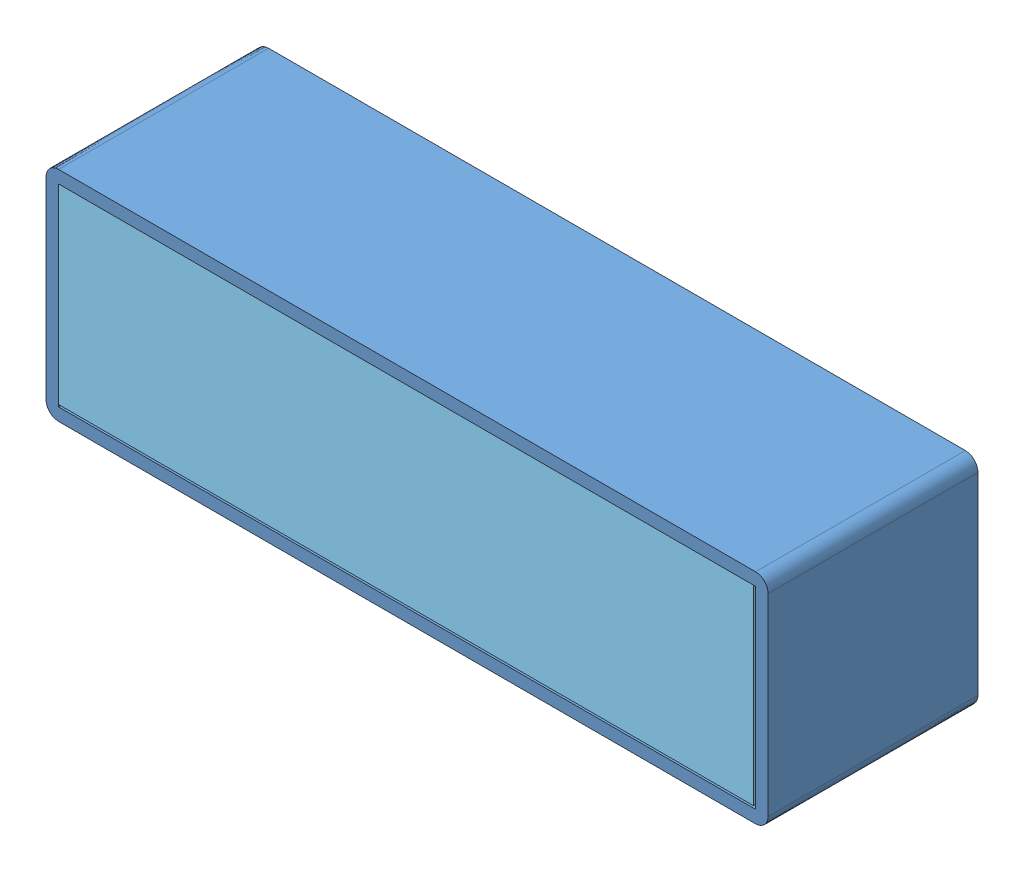
SolidWorks assembly miniAWTRIX, configuration Default. Lengths in mm.
Overall size (172 52 50).
7 component instances, 7 part files, 11 mates.
Components (placement in the parent):
- miniAWTRIX_外壳_壳体-1: miniAWTRIX_外壳_壳体 [默认] at (99.8338 57.2825 83.8628) size (172 52 50)
- miniAWTRIX_PCB-1: miniAWTRIX_PCB [默认] at (60.3647 36.2851 124.7743) size (165.5 45.5 2.82)
- miniAWTRIX_栅格-1: miniAWTRIX_栅格 [默认] at (90.8819 40.7854 124.3628) size (165.5 45.5 4.5)
- miniAWTRIX_匀光板-1: miniAWTRIX_匀光板 [Default] at (173.995 73.539 128.8628) size (165.5 45.5 0.5)
- miniAWTRIX_前面板-1: miniAWTRIX_前面板 [Default] at (173.995 73.7015 132.3628) size (165.5 45.5 1.5)
- miniAWTRIX_MotherBoard-2: miniAWTRIX_MotherBoard [Default] at (30.7417 78.9871 51.8628) x (1 0 0) z (0 -1 0) size (87.57 36.49 16.53)
- miniAWTRIX_后盖-1: miniAWTRIX_后盖 [Default] at (155.5725 64.3667 83.8628) x (-1 0 0) z (0 0 1) size (165 45 38)
Mates (geometry in assembly coordinates):
- 重合1: coincident: line of miniAWTRIX_外壳_壳体-1 through (60.4917 39.2671 124.3628) axis (0 1 0); line of miniAWTRIX_PCB-1 through (60.4917 85.2671 124.3628) axis (0 -1 0)
- 重合2: coincident: plane of miniAWTRIX_外壳_壳体-1 through (99.8338 85.2671 124.3628) normal (0 -1 0); line of miniAWTRIX_PCB-1 through (225.9917 85.2671 124.3628) axis (-1 0 0)
- 重合3: coincident: line of miniAWTRIX_外壳_壳体-1 through (226.4917 39.2671 124.3628) axis (0 1 0); line of miniAWTRIX_栅格-1 through (226.4917 84.7671 124.3628) axis (0 -1 0)
- 重合4: coincident: plane of miniAWTRIX_外壳_壳体-1 through (99.8338 39.2671 124.3628) normal (0 1 0); line of miniAWTRIX_栅格-1 through (60.9917 39.2671 128.8628) axis (1 0 0)
- 重合6: coincident: plane of miniAWTRIX_栅格-1 through (90.8819 40.7854 128.8628) normal (0 0 1); plane of miniAWTRIX_匀光板-1 through (173.995 73.539 128.8628) normal (0 0 -1)
- 重合7: coincident: plane of miniAWTRIX_外壳_壳体-1 through (60.4917 57.2825 124.3628) normal (1 0 0); line of miniAWTRIX_匀光板-1 through (60.4917 85.1046 129.3628) axis (0 -1 0)
- 重合8: coincident: line of miniAWTRIX_外壳_壳体-1 through (60.4917 39.2671 133.8628) axis (0 1 0); line of miniAWTRIX_前面板-1 through (60.4917 85.2671 133.8628) axis (0 -1 0)
- 重合9: coincident: line of miniAWTRIX_外壳_壳体-1 through (226.4917 85.2671 133.8628) axis (-1 0 0); line of miniAWTRIX_前面板-1 through (225.9917 85.2671 133.8628) axis (-1 0 0)
- 同心1: concentric: circle of miniAWTRIX_MotherBoard-2; circle of miniAWTRIX_后盖-1
- 重合10: coincident: line of miniAWTRIX_MotherBoard-2 through (142.9632 78.7671 85.3689) axis (1 0 0); plane of miniAWTRIX_后盖-1 through (155.5725 78.7671 86.8628) normal (0 -1 0)
- 同心5: concentric: circle of miniAWTRIX_外壳_壳体-1; circle of miniAWTRIX_后盖-1
